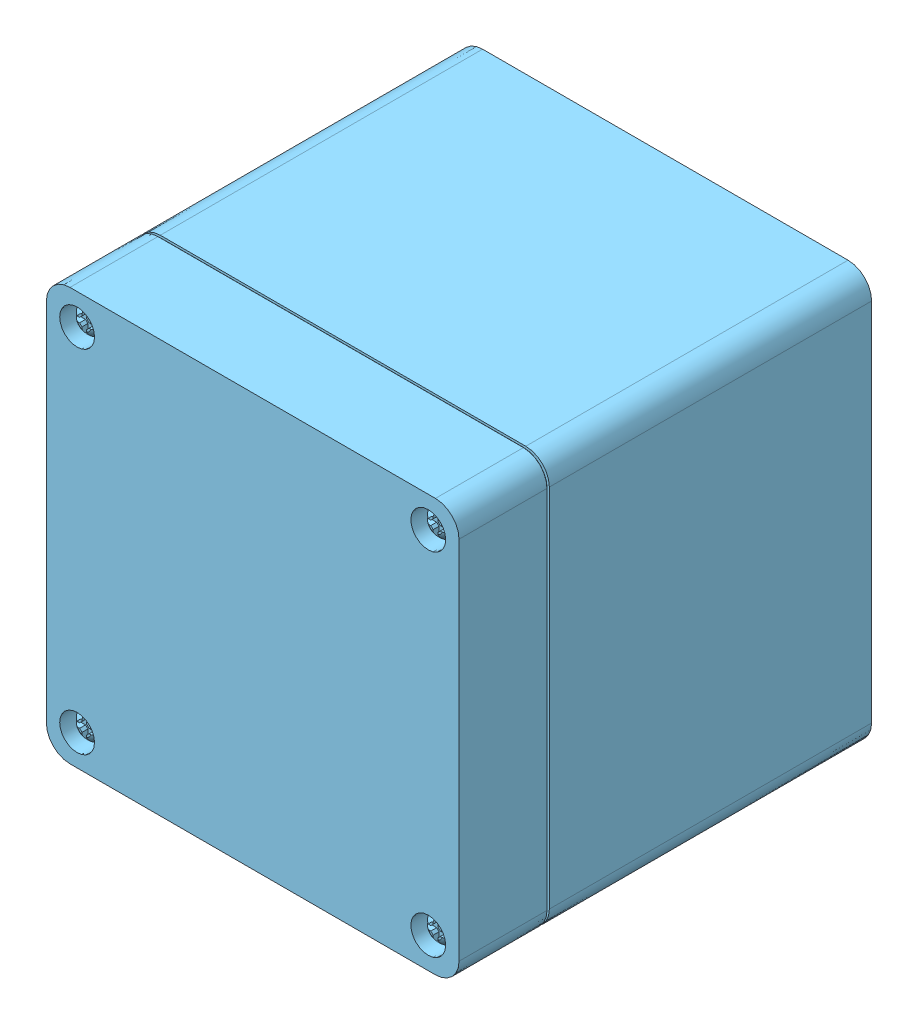
SolidWorks assembly CameraAssembly2, configuration Default. Lengths in mm.
Overall size (93.62 137.91 89.04).
11 component instances, 9 part files, 25 mates.
Components (placement in the parent):
- Camera-1: Camera [Default] at origin size (50 58 30)
- Lens MountV3-1: Lens MountV3 [Default] at (0.0011 0.0011 32.5) x (0.707107 0.707107 0) z (0.707107 -0.707107 0) size (64.2 30.8 68.2)
- 90591A265_Zinc-Plated Steel Hex Nut-2: 90591A265_Zinc-Plated Steel Hex Nut [90591A265] at (-21.3172 4.8011 35.5) x (0.971392 0 0.237482) z (0 1 0) size (4 4.62 1.87)
- 91290A017_Black-Oxide Alloy Steel Socket Head Screw-2: 91290A017_Black-Oxide Alloy Steel Socket Head Screw [91290A017] at (-21.3172 0.0011 35.5) x (1 0 0) z (0 -1 0) size (3.8 3.8 12.09)
- Enclosure2-1: Enclosure2 [4058N13] at (0 0 58.3889) size (88.9 88.9 88.9)
- Gland2-1: Gland2 [69915K48] at (-19 -37.1 -2.5) x (1 0 0) z (0 1 0) size (18.18 16.4 62.56)
- 93395A277_316 Stainless Steel Hex Drive Flat Head Screw-1: 93395A277_316 Stainless Steel Hex Drive Flat Head Screw [93395A277] at (-21 21.0021 -13.1997) x (0.451918 0.89206 0) z (0 0 -1) size (8 8 40.56)
- 93395A277_316 Stainless Steel Hex Drive Flat Head Screw-3: 93395A277_316 Stainless Steel Hex Drive Flat Head Screw [93395A277] at (21.0021 -21 -13.1997) x (-0.097687 -0.995217 0) z (0 0 -1) size (8 8 40.56)
- 90591A255_Zinc-Plated Steel Hex Nut-1: 90591A255_Zinc-Plated Steel Hex Nut [90591A255] at (-21 21.0021 20.1) x (0.998846 0.048026 0) z (0 0 1) size (7 8.08 3.52)
- 90591A255_Zinc-Plated Steel Hex Nut-2: 90591A255_Zinc-Plated Steel Hex Nut [90591A255] at (21.0021 -21 20.1) x (0.965926 0.258819 0) z (0 0 1) size (7 8.08 3.52)
- Lens-1: Lens [Default] at (0.0011 0.0011 32.5) x (1 0 0) z (0 -1 0) size (25 5.06 25)
Mates (geometry in assembly coordinates):
- Concentric1: concentric aligned: cylinder of Camera-1 through (-21 -21 -12.501) axis (0 0 1) radius 2.4; cylinder of Lens MountV3-1 through (-21 -21 7.7) axis (0 0 1) radius 2.4
- Parallel1: parallel aligned: plane of Camera-1 through (-25 -25 12.5) normal (0 -1 0); plane of Lens MountV3-1 through (0.0011 -3.9989 17.1767) normal (0 -1 0)
- Coincident2: coincident anti-aligned: plane of Camera-1 through (0 0 12.5) normal (0 0 1); plane of Lens MountV3-1 through (-18.2252 -14.8311 12.5) normal (0 0 -1)
- Concentric2: concentric aligned: cylinder of Lens MountV3-1 through (-21.3172 -8.9487 35.5) axis (0 1 0) radius 1.75; cylinder of 91290A017_Black-Oxide Alloy Steel Socket Head Screw-2 through (-21.3172 6.0011 35.5) axis (0 1 0) radius 1.9
- Coincident3: coincident anti-aligned: plane of Lens MountV3-1 through (0.0011 -3.9989 17.1767) normal (0 -1 0); plane of 91290A017_Black-Oxide Alloy Steel Socket Head Screw-2 through (-21.3172 -3.9989 37.3) normal (0 1 0)
- Parallel2: parallel anti-aligned: plane of Lens MountV3-1 through (0.0011 4.0011 17.1767) normal (0 1 0); plane of 90591A265_Zinc-Plated Steel Hex Nut-2 through (-21.3172 4.0011 35.5) normal (0 -1 0)
- Concentric3: concentric aligned: circle of 90591A265_Zinc-Plated Steel Hex Nut-2; circle of 91290A017_Black-Oxide Alloy Steel Socket Head Screw-2
- Coincident6: coincident anti-aligned: plane of Lens MountV3-1 through (0.0011 4.0011 17.1767) normal (0 1 0); plane of 90591A265_Zinc-Plated Steel Hex Nut-2 through (-21.3172 4.0011 35.5) normal (0 -1 0)
- Width1: width anti-aligned: plane of Camera-1 through (-25 25 12.5) normal (0 1 0); plane of Enclosure2-1 through (-25 -25 12.5) normal (0 -1 0); plane of Camera-1 through (-31.75 41.4503 -132.7388) normal (0 -1 0); plane of Enclosure2-1 through (31.75 -41.4503 -132.7388) normal (0 1 0)
- Width2: width aligned: plane of Camera-1 through (-25 25 12.5) normal (-1 0 0); plane of Enclosure2-1 through (25 25 12.5) normal (1 0 0); plane of Camera-1 through (41.4503 21.9507 -132.7388) normal (-1 0 0); plane of Enclosure2-1 through (-41.4503 -21.9507 -132.7388) normal (1 0 0)
- LimitDistance1: limit distance = 0 mm anti-aligned: plane of Camera-1 through (0 0 -12.5) normal (0 0 -1); plane of Enclosure2-1 through (0 0 -12.5) normal (0 0 1)
- Concentric4: concentric aligned: circle of Enclosure2-1; circle of Gland2-1
- Coincident8: coincident anti-aligned: plane of Enclosure2-1 through (-44.45 -44.45 -15.4997) normal (0 -1 0); plane of Gland2-1 through (-19 -44.45 -10.7) normal (0 1 0)
- Tangent7: tangent: circle of 93395A277_316 Stainless Steel Hex Drive Flat Head Screw-3; torus of 9262K102_Oil-Resistant Buna-N O-Ring-3
- Concentric7: concentric aligned: circle of 93395A277_316 Stainless Steel Hex Drive Flat Head Screw-3; circle of 9262K102_Oil-Resistant Buna-N O-Ring-3
- Concentric8: concentric aligned: cylinder of Lens MountV3-1 through (-21 21.0021 7.699) axis (0 0 1) radius 2.25; circle of 93395A277_316 Stainless Steel Hex Drive Flat Head Screw-1
- Coincident9: coincident aligned: plane of Enclosure2-1 through (0 0 -15.4997) normal (0 0 -1); plane of 93395A277_316 Stainless Steel Hex Drive Flat Head Screw-1 through (-21 21.0021 -15.4997) normal (0 0 -1)
- Concentric9: concentric aligned: cylinder of Lens MountV3-1 through (21.0021 -21 7.699) axis (0 0 1) radius 2.25; circle of 93395A277_316 Stainless Steel Hex Drive Flat Head Screw-3
- Coincident10: coincident aligned: plane of Enclosure2-1 through (0 0 -15.4997) normal (0 0 -1); plane of 93395A277_316 Stainless Steel Hex Drive Flat Head Screw-3 through (21.0021 -21 -15.4997) normal (0 0 -1)
- Concentric10: concentric aligned: circle of Lens MountV3-1; circle of 90591A255_Zinc-Plated Steel Hex Nut-2
- Coincident12: coincident anti-aligned: plane of Lens MountV3-1 through (21.0021 -24.3941 18.5) normal (0 0 1); plane of 90591A255_Zinc-Plated Steel Hex Nut-2 through (21.0021 -21 18.5) normal (0 0 -1)
- Concentric11: concentric anti-aligned: circle of Lens MountV3-1; circle of 90591A255_Zinc-Plated Steel Hex Nut-1
- Coincident13: coincident anti-aligned: plane of Lens MountV3-1 through (-21 24.3963 18.5) normal (0 0 1); plane of 90591A255_Zinc-Plated Steel Hex Nut-1 through (-21 21.0021 18.5) normal (0 0 -1)
- Coincident14: coincident aligned: plane of Lens MountV3-1 through (-7.1761 10.5723 32.5) normal (0 0 -1); plane of Lens-1 through (0.0011 0.0011 32.5) normal (0 0 -1)
- Concentric12: concentric aligned: circle of Lens MountV3-1; circle of Lens-1
